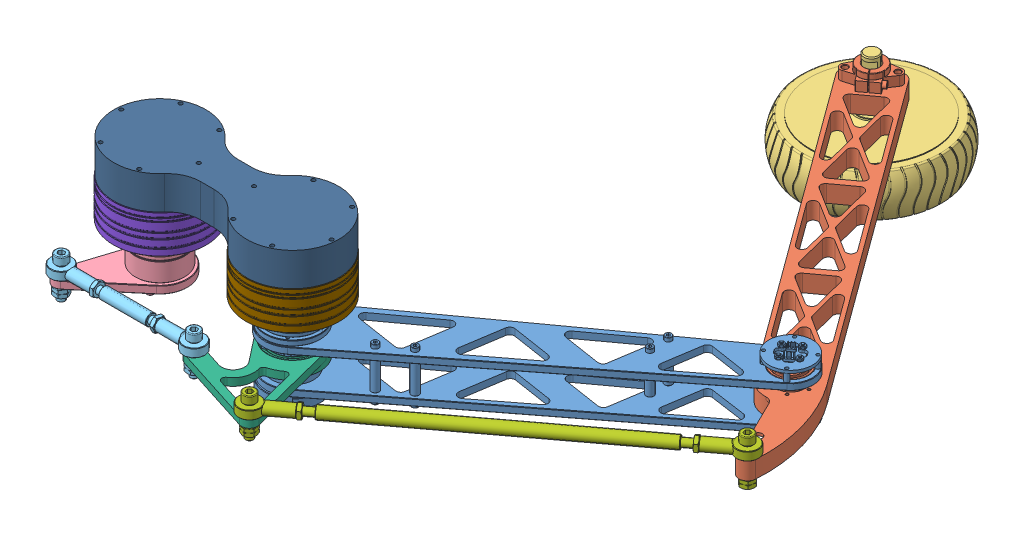
SolidWorks assembly urdf_model, configuration По умолчанию. Lengths in mm.
Overall size (673.37 201 759.45).
10 component instances, 10 part files, 24 mates.
Components (placement in the parent):
- hip_pitch^urdf_model-1: hip_pitch^urdf_model [По умолчанию] x (0.978419 0 -0.206633) z (0.206633 0 0.978419) size (393.52 78 211.65) (virtual)
- knee_pitch^urdf_model-1: knee_pitch^urdf_model [По умолчанию] at (-74.6911 0 -209.8901) x (0.922973 0 0.384864) z (-0.384864 0 0.922973) size (442.96 54 305.38) (virtual)
- ankle_wheel^urdf_model-1: ankle_wheel^urdf_model [По умолчанию] at (64.1964 0 -180.5703) size (172.09 111 172.08) (virtual)
- knee_crank^urdf_model-1: knee_crank^urdf_model [По умолчанию] at (-45.6614 0 103.4419) x (0.922973 0 0.384864) z (-0.384864 0 0.922973) size (58 48.5 110.83) (virtual)
- knee_rod_u^urdf_model-1: knee_rod_u^urdf_model [По умолчанию] at (-59.6536 0 -10.5198) x (0.906308 0 -0.422618) z (0.422618 0 0.906308) size (149.88 43 82.17) (virtual)
- knee_ternary^urdf_model-1: knee_ternary^urdf_model [По умолчанию] x (0.922973 0 0.384864) z (-0.384864 0 0.922973) size (112.51 14 110.83) (virtual)
- knee_rod_b^urdf_model-1: knee_rod_b^urdf_model [По умолчанию] at (-43.1213 0 40.8654) x (0.978419 0 -0.206633) z (0.206633 0 0.978419) size (363.02 48 181.15) (virtual)
- Актуатор АК10-9_00^urdf_model-1: Актуатор АК10-9_00^urdf_model [По умолчанию] at (-140 0.05 0) x (0 -1 0) z (-0.496859 0 0.867831) size (61.7 98 98) (virtual)
- hip_pitch_actuator^urdf_model-1: hip_pitch_actuator^urdf_model [По умолчанию] at origin size (98 61.7 98) (virtual)
- base^urdf_model-1: base^urdf_model [По умолчанию] x (0.906308 0 -0.422618) z (0.422618 0 0.906308) size (223.88 35 156.17) (virtual)
Mates (geometry in assembly coordinates):
- Parallel1: parallel aligned: plane of base^urdf_model-1 through (-95.8157 50.55 20) normal (0 0 1)
- Parallel2: parallel aligned: plane of base^urdf_model-1 through (-70 85.55 0) normal (0 1 0)
- Concentric1: concentric anti-aligned: cylinder of hip_pitch_actuator^urdf_model-1 through (0 64.835 0) axis (0 -1 0) radius 49; cylinder of base^urdf_model-1 through (0 50.55 0) axis (0 1 0) radius 48.5
- Coincident5: coincident anti-aligned: plane of hip_pitch_actuator^urdf_model-1 through (0 50.55 0) normal (0 1 0); plane of base^urdf_model-1 through (-70 50.55 0) normal (0 -1 0)
- Concentric2: concentric anti-aligned: cylinder of Актуатор АК10-9_00^urdf_model-1 through (-140 64.835 0) axis (0 -1 0) radius 49; cylinder of base^urdf_model-1 through (-140 50.55 0) axis (0 1 0) radius 48.5
- Coincident6: coincident anti-aligned: plane of Актуатор АК10-9_00^urdf_model-1 through (-140 50.55 0) normal (0 1 0); plane of base^urdf_model-1 through (-70 50.55 0) normal (0 -1 0)
- Coincident9: coordinate: unknown of hip_pitch_actuator^urdf_model-1
- Concentric3: concentric anti-aligned: cylinder of knee_pitch^urdf_model-1 through (68.0009 -14.45 -542.2056) axis (0 -1 0) radius 14; cylinder of ankle_wheel^urdf_model-1 through (68.0009 -29.95 -542.2056) axis (0 1 0) radius 8
- Distance1: distance = 10 mm aligned: plane of knee_pitch^urdf_model-1 through (68.0009 -14.45 -542.2056) normal (0 1 0); plane of ankle_wheel^urdf_model-1 through (68.0009 -4.45 -542.2056) normal (0 1 0)
- Concentric4: concentric anti-aligned: cylinder of hip_pitch^urdf_model-1 through (300.0046 -62.95 -224.9939) axis (0 1 0) radius 18.5; cylinder of knee_pitch^urdf_model-1 through (300.0046 -240.1086 -224.9939) axis (0 -1 0) radius 14
- Distance2: distance = 7.5 mm anti-aligned: plane of knee_pitch^urdf_model-1 through (300.0046 -30.45 -224.9939) normal (0 1 0); plane of hip_pitch^urdf_model-1 through (0 -22.95 0) normal (0 -1 0)
- Concentric5: concentric anti-aligned: cylinder of hip_pitch^urdf_model-1 through (0 -480.6294 0) axis (0 -1 0) radius 16; cylinder of knee_ternary^urdf_model-1 through (0 -38.45 0) axis (0 1 0) radius 29
- Distance3: distance = 7.5 mm anti-aligned: plane of knee_ternary^urdf_model-1 through (0 -30.45 0) normal (0 1 0); plane of hip_pitch^urdf_model-1 through (0 -22.95 0) normal (0 -1 0)
- Concentric6: concentric anti-aligned: cylinder of hip_pitch^urdf_model-1 through (0 -22.95 0) axis (0 1 0) radius 30; cylinder of hip_pitch_actuator^urdf_model-1 through (0 64.835 0) axis (0 -1 0) radius 49
- Concentric7: concentric anti-aligned: cylinder of knee_rod_u^urdf_model-1 through (-41.7427 -19.95 62.3101) axis (0 -1 0) radius 11.5; cylinder of knee_ternary^urdf_model-1 through (-41.7427 -38.45 62.3101) axis (0 1 0) radius 8.25
- Coincident13: coincident anti-aligned: plane of knee_rod_u^urdf_model-1 through (-39.9677 -38.45 66.1166) normal (0 1 0); plane of knee_ternary^urdf_model-1 through (0 -38.45 0) normal (0 -1 0)
- Concentric8: concentric aligned: cylinder of knee_crank^urdf_model-1 through (-181.7427 -38.45 62.3101) axis (0 1 0) radius 8.25; cylinder of knee_rod_u^urdf_model-1 through (-181.7427 21.3 62.3101) axis (0 1 0) radius 4
- Coincident14: coincident anti-aligned: plane of knee_crank^urdf_model-1 through (-140 -38.45 0) normal (0 -1 0); plane of knee_rod_u^urdf_model-1 through (-179.9677 -38.45 66.1166) normal (0 1 0)
- Concentric9: concentric anti-aligned: cylinder of knee_crank^urdf_model-1 through (-140 -30.45 0) axis (0 1 0) radius 26; cylinder of Актуатор АК10-9_00^urdf_model-1 through (-140 64.835 0) axis (0 -1 0) radius 49
- Coincident15: coincident anti-aligned: plane of knee_crank^urdf_model-1 through (-140 0.05 0) normal (0 1 0); plane of Актуатор АК10-9_00^urdf_model-1 through (-140 0.05 0) normal (0 -1 0)
- Concentric10: concentric aligned: cylinder of knee_ternary^urdf_model-1 through (44.1211 -38.45 89.7403) axis (0 1 0) radius 8.25; cylinder of knee_rod_b^urdf_model-1 through (44.1211 21.3 89.7403) axis (0 1 0) radius 4
- Coincident16: coincident anti-aligned: plane of knee_ternary^urdf_model-1 through (0 -38.45 0) normal (0 -1 0); plane of knee_rod_b^urdf_model-1 through (44.9889 -38.45 93.8497) normal (0 1 0)
- Concentric11: concentric aligned: cylinder of knee_pitch^urdf_model-1 through (344.1257 -48.45 -135.2535) axis (0 1 0) radius 9; cylinder of knee_rod_b^urdf_model-1 through (344.1257 21.3 -135.2535) axis (0 1 0) radius 4
- Angle1: planar angle = 1.570796 rad anti-aligned: plane of hip_pitch^urdf_model-1 through (-16.5295 -62.95 -22.6003) normal (-0.59034 0 -0.807154); plane of knee_pitch^urdf_model-1 through (277.8079 -48.45 -208.7595) normal (-0.807154 0 0.59034)
